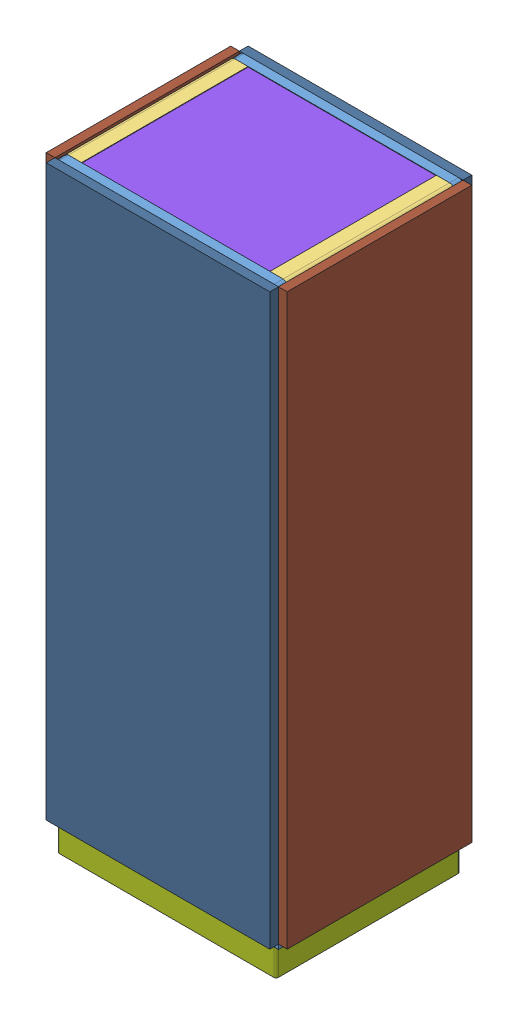
SolidWorks assembly M3DD Assembly - Copy, configuration Default. Lengths in mm.
Overall size (698.5 1739.9 585.8).
24 component instances, 13 part files, 67 mates.
Components (placement in the parent):
- sides-1: sides [Default] at origin size (647.7 1663.7 42.93)
- mounting plate 1-1: mounting plate 1 [Default] at (1.397 226.822 11.43) size (641.35 190.5 12.7)
- mounting plate 1-2: mounting plate 1 [Default] at (1.397 -281.178 11.43) size (641.35 190.5 12.7)
- crossbeam top-1: crossbeam top [Default] at (-323.85 831.85 -482.6) x (0 -1 0) z (0 0 1) size (50.8 50.8 482.6)
- crossbeam top-2: crossbeam top [Default] at (323.85 831.85 -482.6) x (-1 0 0) z (0 0 1) size (50.8 50.8 482.6)
- sides-3: sides [Default] at (0 0 -482.6) x (-1 0 0) z (0 0 -1) size (647.7 1663.7 42.93)
- mounting plate 1-3: mounting plate 1 [Default] at (1.397 226.822 -494.03) x (-1 0 0) z (0 0 -1) size (641.35 190.5 12.7)
- mounting plate 1-4: mounting plate 1 [Default] at (1.397 -281.178 -494.03) x (-1 0 0) z (0 0 -1) size (641.35 190.5 12.7)
- mounting plate 2-2: mounting plate 2 [Default] at (1.397 740.537 9.6139) x (-1 0 0) z (0 0 1) size (641.35 107.95 14.52)
- mounting plate 2-3: mounting plate 2 [Default] at (1.397 740.537 -492.2139) x (1 0 0) z (0 0 -1) size (641.35 107.95 14.52)
- mounting plate 3-1: mounting plate 3 [Default] at (1.397 -776.097 9.6139) size (641.35 107.95 31.53)
- mounting plate 3-2: mounting plate 3 [Default] at (1.397 -776.097 -492.2139) x (-1 0 0) z (0 0 -1) size (641.35 107.95 31.53)
- crossbeam bottom-1: crossbeam bottom [Default] at (-323.85 -806.45 -241.3) x (0 0 -1) z (1 0 0) size (482.6 50.8 69.85)
- crossbeam bottom-2: crossbeam bottom [Default] at (323.85 -806.45 -241.3) x (0 0 1) z (-1 0 0) size (482.6 50.8 69.85)
- base-2: base [Default] at (0.0443 -831.85 -240.03) x (0 0 -1) z (0 -1 0) size (533.4 635 76.2)
- base plate-3: base plate [Default] at (4.458 -808.9265 -240.4999) x (1 0 0) z (0 -1 0) size (546.1 495.3 3.17) (hidden)
- 21x19 plywood-1: 21x19 plywood [Default] at (0 830.3283 -241.3) x (0 0 1) z (0 -1 0) size (482.6 546.1 12.7)
- 20x24 sheet metal-1: 20x24 sheet metal [Default] at (-4.572 812.1673 -237.2741) x (1 0 0) z (0 1 0) size (609.6 508 3.17)
- foam 1-1: foam 1 [Default] at (0.15 6.85 51.638) x (-1 0 0) z (0 0 -1) size (648 1650 25.4)
- foam 1-2: foam 1 [Default] at (-0.15 6.85 -534.162) size (648 1650 25.4)
- foam 2-1: foam 2 [Default] at (323.85 6.85 -241.262) x (0 0 -1) z (1 0 0) size (535 1650 25.4)
- foam 2-2: foam 2 [Default] at (-323.85 6.85 -241.262) x (0 0 1) z (-1 0 0) size (535 1650 25.4)
- heater-1: heater [Default] at (-180.467 812.1673 -362.3691) x (0 0 -1) z (-1 0 0) size (80.01 12.7 80.01)
- heater-2: heater [Default] at (180.467 812.1673 -120.2309) x (1 0 0) z (0 0 -1) size (80.01 12.7 80.01)
Mates (geometry in assembly coordinates):
- Coincident3: coincident anti-aligned: plane of sides-1 through (0 0 24.13) normal (0 0 -1); plane of mounting plate-1 through (1.397 226.822 24.13) normal (0 0 1)
- Coincident4: coincident anti-aligned: plane of sides-1 through (322.072 -831.85 26.162) normal (-1 0 0); plane of mounting plate-1 through (322.072 131.572 24.13) normal (1 0 0)
- Coincident6: coincident anti-aligned: plane of sides-1 through (0 0 24.13) normal (0 0 -1); plane of mounting plate-2 through (1.397 -281.178 24.13) normal (0 0 1)
- Coincident7: coincident anti-aligned: plane of sides-1 through (322.072 -831.85 26.162) normal (-1 0 0); plane of mounting plate-2 through (322.072 -376.428 24.13) normal (1 0 0)
- Coincident10: coincident anti-aligned: plane of sides-1 through (0 0 0) normal (0 0 -1); plane of crossbeam-1 through (-311.15 819.15 0) normal (0 0 1)
- Parallel1: parallel anti-aligned: line of sides-1 through (622.3 -311.15 831.85) axis (0 1 0); line of crossbeam-1 through (38.1 -273.05 831.85) axis (0 -1 0)
- Concentric2: concentric anti-aligned: circle of sides-1; circle of crossbeam-1
- Coincident24: coincident anti-aligned: plane of sides-1 through (0 0 0) normal (0 0 -1); plane of crossbeam-2 through (311.15 819.15 0) normal (0 0 1)
- Concentric9: concentric anti-aligned: circle of sides-1; circle of crossbeam-2
- Coincident25: coincident anti-aligned: line of sides-1 through (622.3 -311.15 831.85) axis (0 1 0); line of crossbeam-2 through (38.1 311.15 831.85) axis (0 -1 0)
- Coincident26: coincident anti-aligned: plane of crossbeam-1 through (-311.15 819.15 -482.6) normal (0 0 -1); plane of sides-3 through (0 0 -482.6) normal (0 0 1)
- Concentric10: concentric aligned: circle of crossbeam-2; circle of sides-3
- Coincident27: coincident aligned: circle of crossbeam-1; circle of sides-3
- Coincident28: coincident anti-aligned: plane of sides-3 through (0 0 -506.73) normal (0 0 1); plane of mounting plate-3 through (1.397 226.822 -506.73) normal (0 0 -1)
- Coincident29: coincident anti-aligned: plane of sides-3 through (322.072 -831.85 -508.762) normal (-1 0 0); plane of mounting plate-3 through (322.072 131.572 -506.73) normal (1 0 0)
- Coincident30: coincident anti-aligned: plane of sides-3 through (0 0 -506.73) normal (0 0 1); plane of mounting plate-4 through (1.397 -281.178 -506.73) normal (0 0 -1)
- Coincident31: coincident anti-aligned: plane of sides-3 through (322.072 -831.85 -508.762) normal (-1 0 0); plane of mounting plate-4 through (322.072 -376.428 -506.73) normal (1 0 0)
- Distance1: distance = 508 mm anti-aligned: plane of sides-1 through (-323.85 830.072 26.162) normal (0 -1 0); plane of mounting plate-1 through (-319.278 322.072 24.13) normal (0 1 0)
- Distance2: distance = 1016 mm anti-aligned: plane of sides-1 through (-323.85 830.072 26.162) normal (0 -1 0); plane of mounting plate-2 through (-319.278 -185.928 24.13) normal (0 1 0)
- Distance3: distance = 508 mm anti-aligned: plane of sides-3 through (323.85 830.072 -508.762) normal (0 -1 0); plane of mounting plate-3 through (322.072 322.072 -506.73) normal (0 1 0)
- Distance4: distance = 1016 mm anti-aligned: plane of sides-3 through (323.85 830.072 -508.762) normal (0 -1 0); plane of mounting plate-4 through (322.072 -185.928 -506.73) normal (0 1 0)
- Coincident33: coincident anti-aligned: plane of sides-1 through (0 0 24.13) normal (0 0 -1); plane of mounting plate 2-2 through (1.397 740.537 24.13) normal (0 0 1)
- Distance5: distance = 35.56 mm anti-aligned: plane of sides-1 through (-323.85 830.072 26.162) normal (0 -1 0); plane of mounting plate 2-2 through (322.072 794.512 24.13) normal (0 1 0)
- Coincident35: coincident anti-aligned: plane of sides-1 through (322.072 -831.85 26.162) normal (-1 0 0); plane of mounting plate 2-2 through (322.072 794.512 24.13) normal (1 0 0)
- Coincident36: coincident anti-aligned: plane of sides-3 through (0 0 -506.73) normal (0 0 1); plane of mounting plate 2-3 through (1.397 740.537 -506.73) normal (0 0 -1)
- Distance6: distance = 35.56 mm anti-aligned: plane of sides-3 through (323.85 830.072 -508.762) normal (0 -1 0); plane of mounting plate 2-3 through (-319.278 794.512 -506.73) normal (0 1 0)
- Coincident39: coincident anti-aligned: plane of sides-3 through (322.072 -831.85 -508.762) normal (-1 0 0); plane of mounting plate 2-3 through (322.072 794.512 -506.73) normal (1 0 0)
- Coincident40: coincident anti-aligned: plane of sides-1 through (0 0 24.13) normal (0 0 -1); plane of mounting plate 3-1 through (1.397 -776.097 24.13) normal (0 0 1)
- Coincident41: coincident anti-aligned: plane of sides-1 through (322.072 -831.85 26.162) normal (-1 0 0); plane of mounting plate 3-1 through (322.072 -830.072 24.13) normal (1 0 0)
- Coincident42: coincident anti-aligned: plane of sides-1 through (-323.85 -830.072 26.162) normal (0 1 0); plane of mounting plate 3-1 through (-319.278 -830.072 24.13) normal (0 -1 0)
- Coincident43: coincident anti-aligned: plane of sides-3 through (0 0 -506.73) normal (0 0 1); plane of mounting plate 3-2 through (1.397 -776.097 -506.73) normal (0 0 -1)
- Coincident44: coincident anti-aligned: plane of sides-3 through (322.072 -831.85 -508.762) normal (-1 0 0); plane of mounting plate 3-2 through (322.072 -830.072 -506.73) normal (1 0 0)
- Coincident45: coincident anti-aligned: plane of sides-3 through (323.85 -830.072 -508.762) normal (0 1 0); plane of mounting plate 3-2 through (322.072 -830.072 -506.73) normal (0 -1 0)
- Coincident46: coincident aligned: plane of sides-3 through (-323.85 -831.85 -508.762) normal (-1 0 0); plane of crossbeam bottom-1 through (-323.85 -806.45 -241.3) normal (-1 0 0)
- Coincident47: coincident anti-aligned: plane of sides-1 through (0 0 0) normal (0 0 -1); plane of crossbeam bottom-1 through (-254 -831.85 0) normal (0 0 1)
- Coincident48: coincident aligned: plane of sides-1 through (-323.85 -831.85 26.162) normal (0 -1 0); plane of crossbeam bottom-1 through (-254 -831.85 0) normal (0 -1 0)
- Coincident49: coincident aligned: plane of sides-1 through (323.85 -831.85 26.162) normal (1 0 0); plane of crossbeam bottom-2 through (323.85 -806.45 -241.3) normal (1 0 0)
- Coincident50: coincident anti-aligned: plane of sides-3 through (0 0 -482.6) normal (0 0 1); plane of crossbeam bottom-2 through (254 -831.85 -482.6) normal (0 0 -1)
- Coincident51: coincident aligned: plane of sides-1 through (-323.85 -831.85 26.162) normal (0 -1 0); plane of crossbeam bottom-2 through (254 -831.85 -482.6) normal (0 -1 0)
- Coincident53: coincident anti-aligned: plane of crossbeam bottom-1 through (-254 -831.85 0) normal (0 -1 0); plane of base-2 through (0.0443 -831.85 -240.03) normal (0 1 0)
- Parallel3: parallel anti-aligned: line of crossbeam bottom-1 through (-323.85 -829.31 -482.6) axis (0 0 1); line of base-2 through (-317.4557 -831.85 20.32) axis (0 0 -1)
- Coincident54: coincident aligned: plane of mounting plate 3-2 through (1.397 -776.097 -506.73) normal (0 0 -1); plane of base-2 through (-317.4557 -908.05 -506.73) normal (0 0 -1)
- Coincident91: coincident anti-aligned: plane of sides-3 through (-270.336 817.6283 -465.836) normal (0 1 0); plane of 21x19 plywood-1 through (0 817.6283 -241.3) normal (0 -1 0)
- Coincident92: coincident anti-aligned: plane of sides-3 through (0 0 -482.6) normal (0 0 1); plane of 21x19 plywood-1 through (273.05 817.6283 -482.6) normal (0 0 -1)
- Coincident93: coincident anti-aligned: plane of crossbeam top-2 through (273.05 831.85 0) normal (-1 0 0); plane of 21x19 plywood-1 through (273.05 817.6283 -482.6) normal (1 0 0)
- Coincident109: coincident anti-aligned: plane of sides-3 through (-295.736 815.3423 -506.73) normal (0 -1 0); plane of 20x24 sheet metal-1 through (-4.572 815.3423 -237.2741) normal (0 1 0)
- Distance24: distance = 12.7 mm anti-aligned: plane of mounting plate 2-3 through (1.397 740.537 -503.9741) normal (0 0 1); plane of 20x24 sheet metal-1 through (-309.372 815.3423 -491.2741) normal (0 0 -1)
- Distance23: distance = 12.7 mm anti-aligned: plane of crossbeam top-1 through (-322.072 819.15 0) normal (1 0 0); plane of 20x24 sheet metal-1 through (-309.372 815.3423 16.7259) normal (-1 0 0)
- Distance30: distance = 14.224 mm anti-aligned: plane of base plate-3 through (-268.592 -812.1015 7.1501) normal (0 0 1); plane of mounting plate 3-1 through (1.397 -776.097 21.3741) normal (0 0 -1)
- Coincident130: coincident aligned: plane of sides-1 through (-323.85 -831.85 26.162) normal (-1 0 0); plane of foam 1-1 through (-323.85 -818.15 26.238) normal (-1 0 0)
- Coincident131: coincident aligned: plane of sides-1 through (-323.85 831.85 26.162) normal (0 1 0); plane of foam 1-1 through (324.15 831.85 26.238) normal (0 1 0)
- Coincident133: coincident aligned: plane of sides-3 through (323.85 831.85 -508.762) normal (0 1 0); plane of foam 1-2 through (-324.15 831.85 -508.762) normal (0 1 0)
- Coincident134: coincident aligned: plane of sides-3 through (323.85 -831.85 -508.762) normal (1 0 0); plane of foam 1-2 through (323.85 -818.15 -508.762) normal (1 0 0)
- Coincident135: coincident anti-aligned: plane of sides-3 through (0 0 -508.762) normal (0 0 -1); plane of foam 1-2 through (-0.15 6.85 -508.762) normal (0 0 1)
- Coincident136: coincident anti-aligned: plane of crossbeam top-2 through (323.85 819.15 0) normal (1 0 0); plane of foam 2-1 through (323.85 6.85 -241.262) normal (-1 0 0)
- Distance31: distance = 25.4 mm aligned: plane of foam 1-2 through (-0.15 6.85 -534.162) normal (0 0 -1); plane of foam 2-1 through (349.25 -818.15 -508.762) normal (0 0 -1)
- Coincident138: coincident aligned: plane of foam 1-2 through (-324.15 831.85 -508.762) normal (0 1 0); plane of foam 2-1 through (349.25 831.85 26.238) normal (0 1 0)
- Coincident139: coincident anti-aligned: plane of crossbeam top-1 through (-323.85 819.15 0) normal (-1 0 0); plane of foam 2-2 through (-323.85 6.85 -241.262) normal (1 0 0)
- Coincident140: coincident aligned: plane of foam 2-1 through (349.25 -818.15 -508.762) normal (0 0 -1); plane of foam 2-2 through (-349.25 -818.15 -508.762) normal (0 0 -1)
- Coincident141: coincident aligned: plane of foam 1-2 through (-324.15 831.85 -508.762) normal (0 1 0); plane of foam 2-2 through (-349.25 831.85 -508.762) normal (0 1 0)
- Coincident145: coincident anti-aligned: plane of foam 1-1 through (0.15 6.85 26.238) normal (0 0 -1); plane of foam 2-2 through (-349.25 -818.15 26.238) normal (0 0 1)
- Coincident155: coincident anti-aligned: plane of 20x24 sheet metal-1 through (-4.572 812.1673 -237.2741) normal (0 -1 0); plane of heater-1 through (-180.467 812.1673 -362.3691) normal (0 1 0)
- Distance32: distance = 101.6 mm anti-aligned: plane of heater-1 through (-220.472 799.4673 -402.3741) normal (0 0 -1); plane of mounting plate 2-3 through (1.397 740.537 -503.9741) normal (0 0 1)
- Distance33: distance = 101.6 mm anti-aligned: plane of heater-1 through (-220.472 799.4673 -322.3641) normal (-1 0 0); plane of crossbeam top-1 through (-322.072 819.15 0) normal (1 0 0)
- Coincident158: coincident anti-aligned: plane of 20x24 sheet metal-1 through (-4.572 812.1673 -237.2741) normal (0 -1 0); plane of heater-2 through (180.467 812.1673 -120.2309) normal (0 1 0)
- Distance34: distance = 101.6 mm anti-aligned: plane of heater-2 through (220.472 799.4673 -160.2359) normal (1 0 0); plane of crossbeam top-2 through (322.072 819.15 0) normal (-1 0 0)
- Distance35: distance = 101.6 mm anti-aligned: plane of heater-2 through (140.462 799.4673 -80.2259) normal (0 0 1); plane of mounting plate 2-2 through (1.397 740.537 21.3741) normal (0 0 -1)
